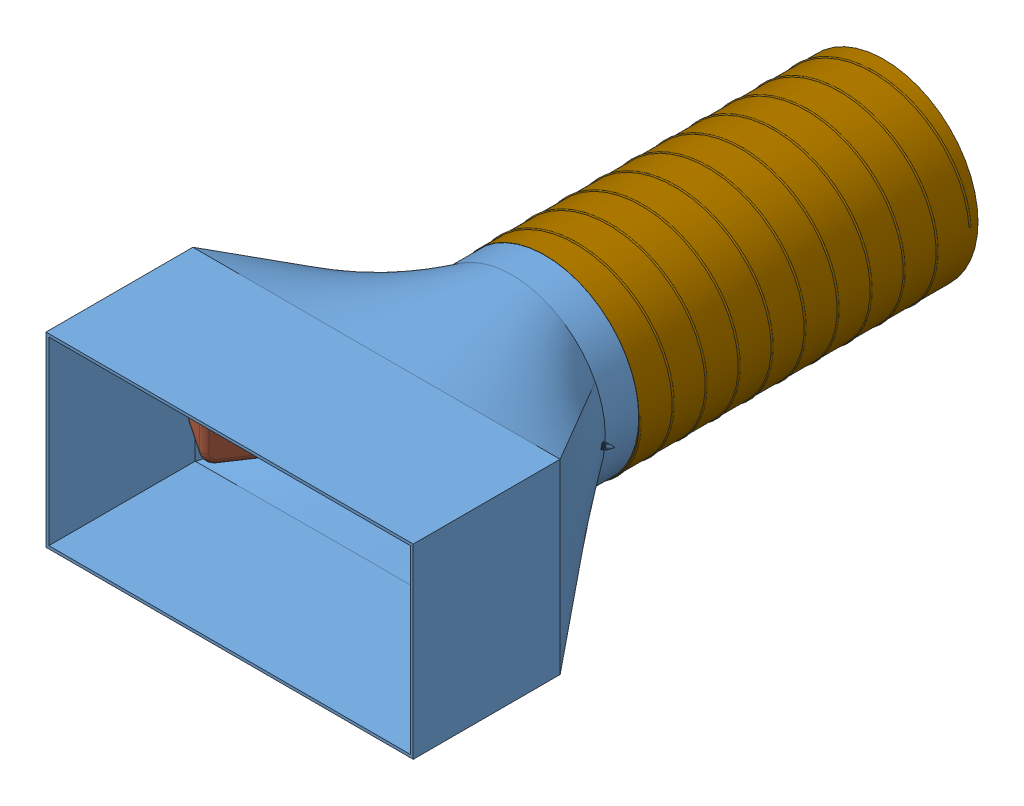
SolidWorks assembly Vent Layout, configuration Default. Lengths in mm.
Overall size (206.38 107.39 367.79).
36 component instances, 21 part files, 13 mates.
Components (placement in the parent):
- Boot 8x4x4-1: Boot 8x4x4 [Default] x (-1 0 0) z (0 1 0) size (206.38 209.55 104.88)
- Damper Assy-1: Damper Assy [Default] at (0 0 -203.2) size (109.18 101.6 116.71)
  - Butterfly Damper, Master-1: Butterfly Damper, Master [Option A] at origin size (109.18 92.71 116.71)
  - Pressure Sensor PCBA-1: Pressure Sensor PCBA [Default] at (-1.016 -4.0521 -52.07) x (0 1 0) z (-1 0 0) size (18 8 4.29)
  - B004N6356S worm-1: B004N6356S worm [Default] at (7.5609 -41.195 -7.2252) x (0.469083 0.855637 -0.218737) z (0.422618 0 0.906308) size (9.8 9.85 19.19)
  - B004N84ZKQ worm gear-1: B004N84ZKQ worm gear [Default] at (0 -40.9829 0) x (0 1 0) z (0.628638 0 0.777698) size (9.99 11.99 11.99)
  - Mabuchi FF-N20WA-9Z190-1: Mabuchi FF-N20WA-9Z190 [Default] at (2.2151 -41.195 -18.6892) x (0.906308 0 -0.422618) z (-0.422618 0 -0.906308) size (25.95 10 52.91)
  - Polyshine F10k-b10kh0-1: Polyshine F10k-b10kh0 [Default] at (0 44.375 4.9) x (-1 0 0) z (0 0 1) size (10.5 5.6 15.2)
  - Custom Gasket-1: Custom Gasket [bent] at (0 0 35.56) x (-1 0 0) z (0 0 -1) size (101.6 101.6 14.48)
- Flex Ducting-1: Flex Ducting [Default] at (0 0 -177.8) size (107.39 107.39 190.5)
- 90190A170_PAN HEAD PHILLIPS SCREW FOR SHEET METAL-5: 90190A170_PAN HEAD PHILLIPS SCREW FOR SHEET METAL [90190A170] at (-49.8345 0 -148.9908) x (0.377871 -0.734223 -0.56403) z (0.83079 0 0.556586) size (7.52 7.52 15.26)
- 90190A170_PAN HEAD PHILLIPS SCREW FOR SHEET METAL-8: 90190A170_PAN HEAD PHILLIPS SCREW FOR SHEET METAL [90190A170] at (49.7899 0 -148.9609) x (-0.520834 0.352619 -0.777426) z (-0.83079 0 0.556586) size (7.52 7.52 15.26)
- Power Module-1: Power Module [Default] at (-68.7685 0 -99.4548) x (0 -1 0) z (-0.556586 0 0.83079) size (79.61 41.85 122.16)
  - Power Module Case-1: Power Module Case [Default] at origin size (64.77 25.4 72.39)
  - Power PCBA-1: Power PCBA [Default] at (-10.16 -7.62 0) x (-1 0 0) z (0 1 0) size (33.74 40 4.78)
  - 801-00020-1: 801-00020 [Default] at (0 2.54 1.27) size (61.87 15.53 67.1)
    - 602-00060-1: 602-00060 [Default] at (0 0 -28.2862) size (61.87 15.53 67.1)
    - 601-00007-1: 601-00007 [Default] at (14.9413 0.4952 26.418) x (-1 0 0) z (0 0.017452 -0.999848) size (20.83 11.61 7.29)
    - 601-00010-2: 601-00010 [Default] at (21.7503 -4.6339 -26.3284) x (1 0 0) z (0 0.017452 0.999848) size (7.94 12.12 7.25)
    - 601-00014-3: 601-00014 [Default] at (-3.3071 1.8398 -26.6943) x (-1 0 0) z (0 0 -1) size (10.97 11.91 7.38)
    - 601-00014-4: 601-00014 [Default] at (25.7107 1.8398 -26.6901) x (-1 0 0) z (0 0 -1) size (10.97 11.91 7.38)
    - 601-00016-2: 601-00016 [Default] at (3.2878 5.966 -26.7675) x (0 0.017452 0.999848) z (-1 0 0) size (2.91 11.43 7.92)
    - 601-00014-5: 601-00014 [Default] at (11.2107 1.8398 -26.6901) x (-1 0 0) z (0 0 -1) size (10.97 11.91 7.38)
    - 601-00014-6: 601-00014 [Default] at (-17.8071 1.8398 -26.6943) x (-1 0 0) z (0 0 -1) size (10.97 11.91 7.38)
    - 601-00007-4: 601-00007 [Default] at (-14.0587 0.4952 26.418) x (-1 0 0) z (0 0.017452 -0.999848) size (20.83 11.61 7.29)
    - 601-00016-4: 601-00016 [Default] at (-25.7122 5.966 -26.7675) x (0 0.017452 0.999848) z (-1 0 0) size (2.91 11.43 7.92)
    - 601-00010-4: 601-00010 [Default] at (-7.2497 -4.6339 -26.3284) x (1 0 0) z (0 0.017452 0.999848) size (7.94 12.12 7.25)
    - 601-00018-1: 601-00018 [Default] at (14.5002 -5.091 0) x (0 0 1) z (-1 0 0) size (59.69 3.45 6.35)
    - 601-00018-2: 601-00018 [Default] at (-14.5002 -5.091 0) x (0 0 1) z (-1 0 0) size (59.69 3.45 6.35)
    - AA Batt-1: AA Batt [Default] at (-21.75 0.635 -1.778) x (-1 0 0) z (0 -1 0) size (13 48.95 13)
    - AA Batt-2: AA Batt [Default] at (-7.366 0.635 1.778) x (1 0 0) z (0 -1 0) size (13 48.95 13)
    - AA Batt-4: AA Batt [Default] at (7.25 0.635 -1.778) x (-1 0 0) z (0 -1 0) size (13 48.95 13)
    - AA Batt-5: AA Batt [Default] at (21.634 0.635 1.778) x (1 0 0) z (0 -1 0) size (13 48.95 13)
  - K&J DH21 Magnet-1: K&J DH21 Magnet [Default] at (-26.7027 -11.9062 -26.3637) size (5.08 1.59 5.08)
  - K&J DH21 Magnet-2: K&J DH21 Magnet [Default] at (24.1434 -11.9062 25.445) x (0.982082 0 -0.188455) z (0.188455 0 0.982082) size (5.08 1.59 5.08)
  - Power Module Wires-1: Power Module Wires [Single Wire] at origin size (37.21 39.1 49.77)
Mates (geometry in assembly coordinates):
- Coincident1: coincident aligned: plane of Boot 8x4x4-1 through (0 0 0) normal (0 0 1); plane of assembly through (0 0 0) normal (0 0 1)
- Coincident2: coincident anti-aligned: plane of Boot 8x4x4-1 through (0 0 0) normal (-1 0 0); plane of assembly through (0 0 0) normal (1 0 0)
- Coincident3: coincident aligned: plane of Boot 8x4x4-1 through (0 0 0) normal (0 1 0); plane of assembly through (0 0 0) normal (0 1 0)
- Coincident4: coincident aligned: plane of Damper Assy-1/Butterfly Damper, Master-1 through (0 0 -203.2) normal (0 1 0); plane of assembly through (0 0 0) normal (0 1 0)
- Coincident5: coincident aligned: plane of Damper Assy-1/Butterfly Damper, Master-1 through (0 0 -203.2) normal (1 0 0); plane of assembly through (0 0 0) normal (1 0 0)
- Distance1: distance = 203.2 mm aligned: plane of Damper Assy-1/Butterfly Damper, Master-1 through (0 0 -203.2) normal (0 0 1); plane of assembly through (0 0 0) normal (0 0 1)
- Coincident23: coincident aligned: plane of Flex Ducting-1 through (0 0 -177.8) normal (0 1 0); plane of assembly through (0 0 0) normal (0 1 0)
- Coincident24: coincident aligned: plane of Flex Ducting-1 through (0 0 -177.8) normal (1 0 0); plane of assembly through (0 0 0) normal (1 0 0)
- Distance2: distance = 177.8 mm aligned: plane of Flex Ducting-1 through (0 0 -177.8) normal (0 0 1); plane of assembly through (0 0 0) normal (0 0 1)
- Coincident30: coincident anti-aligned: plane of ? through (-68.7685 0 -99.4548) normal (0 -1 0); plane of assembly through (0 0 0) normal (0 1 0)
- Concentric8: concentric anti-aligned: cylinder of Damper Assy-1/Butterfly Damper, Master-1 through (-104.9294 0 -185.9015) axis (0.83079 0 0.556586) radius 2.54; circle of 90190A170_PAN HEAD PHILLIPS SCREW FOR SHEET METAL-5
- Concentric9: concentric anti-aligned: cylinder of Damper Assy-1/Butterfly Damper, Master-1 through (104.5684 0 -185.6596) axis (-0.83079 0 0.556586) radius 2.54; circle of 90190A170_PAN HEAD PHILLIPS SCREW FOR SHEET METAL-8
- Distance3: distance = 4.1478 mm anti-aligned: plane of ? through (-59.1739 -32.385 -136.5939) normal (-0.83079 0 -0.556586); plane of Damper Assy-1/Butterfly Damper, Master-1 through (-6.5976 0 -207.6201) normal (0.83079 0 0.556586)
